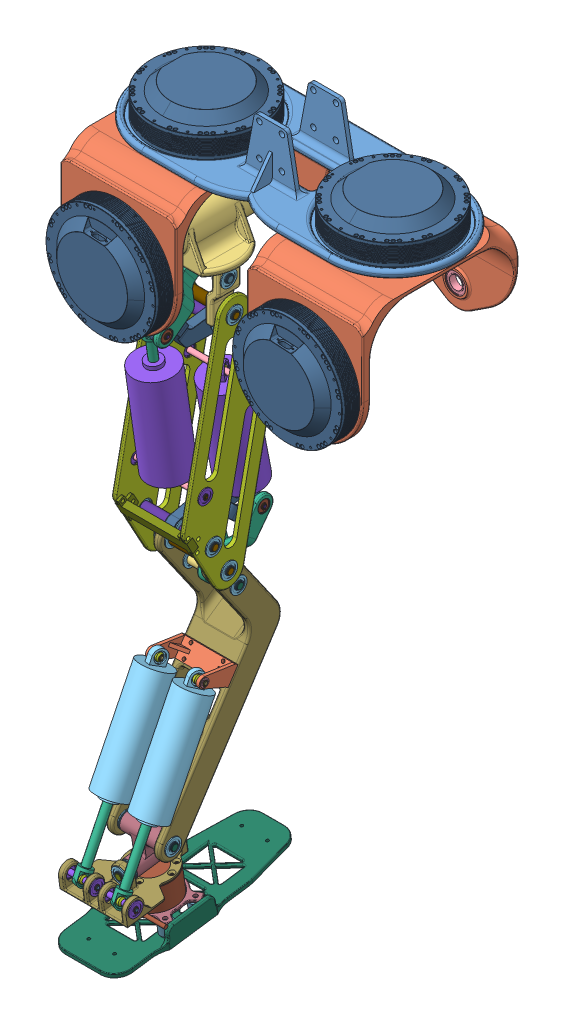
SolidWorks assembly 纯下肢, configuration 默认. Lengths in mm.
Overall size (490 1133.74 383.33).
196 component instances, 46 part files, 330 mates.
Components (placement in the parent):
- 腰部固定座-1: 腰部固定座 [默认] at (0 279.9038 -219.3997) size (490 92.32 200)
- 髋旋转轴-1: 髋旋转轴 [默认] at (-145 260.4038 -219.3997) x (0 0 1) z (-1 0 0) size (243 210 186.66)
- 髋侧摆轴-1: 髋侧摆轴 [默认] at (-145 150.4038 -206.8997) x (-1 0 0) z (0 0 -1) size (125 160 235.8)
- 20mm法兰轴承F63804ZZ-1: 20mm法兰轴承F63804ZZ [默认] at (-145 150.4038 -317.3997) x (0 0 -1) z (0.948831 0.315784 0) size (10 35 35)
- 法兰轴承10_22_6-1: 法兰轴承10_22_6 [默认] at (-190.25 95.4038 -201.6733) x (0 0.630606 0.776103) z (0 0.776103 -0.630606) size (25 6 25)
- 法兰轴承10_22_6-2: 法兰轴承10_22_6 [默认] at (-180.25 45.6778 -206.8997) x (0 -0.265433 0.964129) z (0 0.964129 0.265433) size (25 6 25)
- 法兰轴承10_22_6-3: 法兰轴承10_22_6 [默认] at (-182.25 45.6778 -206.8997) x (0 -0.354717 -0.934974) z (0 0.934974 -0.354717) size (25 6 25)
- 法兰轴承10_22_6-4: 法兰轴承10_22_6 [默认] at (-192.25 95.4038 -201.6733) x (0 -0.95037 0.311121) z (0 -0.311121 -0.95037) size (25 6 25)
- 法兰轴承10_22_6-5: 法兰轴承10_22_6 [默认] at (-99.75 95.4038 -201.6733) x (0 0.630606 0.776103) z (0 -0.776103 0.630606) size (25 6 25)
- 法兰轴承10_22_6-6: 法兰轴承10_22_6 [默认] at (-109.75 45.6778 -206.8997) x (0 -0.265433 0.964129) z (0 -0.964129 -0.265433) size (25 6 25)
- 法兰轴承10_22_6-7: 法兰轴承10_22_6 [默认] at (-107.75 45.6778 -206.8997) x (0 -0.354717 -0.934974) z (0 -0.934974 0.354717) size (25 6 25)
- 法兰轴承10_22_6-8: 法兰轴承10_22_6 [默认] at (-97.75 95.4038 -201.6733) x (0 -0.95037 0.311121) z (0 0.311121 0.95037) size (25 6 25)
- 膝关节U型架-3: 膝关节U型架 [默认] at (-152.25 107.2713 -192.4992) x (1 0 0) z (0 -0.791163 -0.611605) size (56 120 30)
- 法兰轴承10_22_6-9: 法兰轴承10_22_6 [默认] at (-147.75 95.4038 -201.6733) x (0 -0.354389 -0.935098) z (0 0.935098 -0.354389) size (25 6 25)
- 法兰轴承10_22_6-10: 法兰轴承10_22_6 [默认] at (-142.25 95.4038 -201.6733) x (0 -0.969672 -0.244408) z (0 -0.244408 0.969672) size (25 6 25)
- 大腿侧板-1: 大腿侧板 [默认] at (-194.75 -294.2141 -198.324) x (-1 0 0) z (0 0.025223 0.999682) size (6 390 144.2)
- 法兰轴承10_22_6-11: 法兰轴承10_22_6 [默认] at (-196.25 -294.2141 -198.324) x (0 -0.631421 0.77544) z (0 -0.77544 -0.631421) size (25 6 25)
- 法兰轴承5-19-6-1: 法兰轴承5-19-6 [默认] at (-196.25 -176.2424 -161.2878) x (0 -0.967819 -0.251646) z (0 0.251646 -0.967819) size (22 6 22)
- 法兰轴承10_22_6-12: 法兰轴承10_22_6 [默认] at (-196.25 -250.296 -174.4241) x (0 -0.631421 0.77544) z (0 -0.77544 -0.631421) size (25 6 25)
- 法兰轴承5-19-6-2: 法兰轴承5-19-6 [默认] at (-196.25 -73.2936 -243.9107) x (0 -0.631421 0.77544) z (0 -0.77544 -0.631421) size (22 6 22)
- 法兰轴承10_22_6-13: 法兰轴承10_22_6 [默认] at (-196.25 1.7597 -230.7996) x (0 -0.631421 0.77544) z (0 -0.77544 -0.631421) size (25 6 25)
- 法兰轴承10_22_6-14: 法兰轴承10_22_6 [默认] at (-196.25 45.6778 -206.8997) x (0 -0.631421 0.77544) z (0 -0.77544 -0.631421) size (25 6 25)
- 10mm轴114.5mm-1: 10mm轴114.5mm [默认] at (-145 45.6778 -206.8997) x (1 0 0) z (0 0.966924 -0.255065) size (118.9 10 10)
- 大腿侧板-2: 大腿侧板 [默认] at (-89.25 -294.2141 -198.324) x (-1 0 0) z (0 0.025223 0.999682) size (6 390 144.2)
- 法兰轴承10_22_6-19: 法兰轴承10_22_6 [默认] at (-93.75 -294.2141 -198.324) x (0 -0.631421 0.77544) z (0 0.77544 0.631421) size (25 6 25)
- 法兰轴承5-19-6-5: 法兰轴承5-19-6 [默认] at (-93.75 -176.2424 -161.2878) x (0 -0.967819 -0.251646) z (0 -0.251646 0.967819) size (22 6 22)
- 法兰轴承10_22_6-20: 法兰轴承10_22_6 [默认] at (-93.75 -250.296 -174.4241) x (0 -0.631421 0.77544) z (0 0.77544 0.631421) size (25 6 25)
- 法兰轴承5-19-6-6: 法兰轴承5-19-6 [默认] at (-93.75 -73.2936 -243.9107) x (0 -0.631421 0.77544) z (0 0.77544 0.631421) size (22 6 22)
- 法兰轴承10_22_6-21: 法兰轴承10_22_6 [默认] at (-93.75 1.7597 -230.7996) x (0 -0.631421 0.77544) z (0 0.77544 0.631421) size (25 6 25)
- 法兰轴承10_22_6-22: 法兰轴承10_22_6 [默认] at (-93.75 45.6778 -206.8997) x (0 -0.631421 0.77544) z (0 0.77544 0.631421) size (25 6 25)
- 膝关节U型架后侧-3: 膝关节U型架后侧 [默认] at (-152.25 1.6259 -192.216) x (1 0 0) z (0 -0.559181 0.829046) size (38 113.6 87.09)
- 轴承_NSK635-1: 轴承_NSK635 [默认] at (-126 40.3594 -130.4685) x (0 0.759997 0.649927) z (0 -0.649927 0.759997) size (19 6 19)
- 轴承_NSK635-2: 轴承_NSK635 [默认] at (-158 40.3594 -130.4685) x (0 -0.354055 -0.935224) z (0 0.935224 -0.354055) size (19 6 19)
- 轴承_NSK635-3: 轴承_NSK635 [默认] at (-173 40.3594 -130.4685) x (0 0.410059 0.912059) z (0 0.912059 -0.410059) size (19 6 19)
- 轴承_NSK635-4: 轴承_NSK635 [默认] at (-123 40.3594 -130.4685) x (0 0.131283 0.991345) z (0 0.991345 -0.131283) size (19 6 19)
- 法兰轴承10_22_6-27: 法兰轴承10_22_6 [默认] at (-142.25 1.7597 -230.7996) x (0 0.903359 0.428885) z (0 0.428885 -0.903359) size (25 6 25)
- 法兰轴承10_22_6-28: 法兰轴承10_22_6 [默认] at (-147.75 1.7597 -230.7996) x (0 -0.592349 0.805681) z (0 -0.805681 -0.592349) size (25 6 25)
- 法兰轴承10_22_6-29: 法兰轴承10_22_6 [默认] at (-142.25 -250.296 -174.4241) x (0 0.618844 0.785514) z (0 0.785514 -0.618844) size (25 6 25)
- 轴承_NSK635-5: 轴承_NSK635 [默认] at (-158 -263.2782 -281.1374) x (0 0.098206 -0.995166) z (0 0.995166 0.098206) size (19 6 19)
- 轴承_NSK635-6: 轴承_NSK635 [默认] at (-126 -263.2782 -281.1374) x (0 0.098206 -0.995166) z (0 0.995166 0.098206) size (19 6 19)
- 膝关节U型架后侧-4: 膝关节U型架后侧 [默认] at (-152.25 -240.7623 -211.8115) x (1 0 0) z (0 0.74438 -0.667756) size (38 113.6 87.09)
- 法兰轴承10_22_6-30: 法兰轴承10_22_6 [默认] at (-147.75 -250.296 -174.4241) x (0 -0.88858 0.458722) z (0 -0.458722 -0.88858) size (25 6 25)
- 膝关节U型架-4: 膝关节U型架 [默认] at (-152.25 -344.1973 -238.9818) x (1 0 0) z (0 0.601536 0.798846) size (56 120 30)
- 法兰轴承10_22_6-33: 法兰轴承10_22_6 [默认] at (-147.75 -335.1743 -226.9991) x (0 -0.23218 -0.972673) z (0 0.972673 -0.23218) size (25 6 25)
- 法兰轴承10_22_6-34: 法兰轴承10_22_6 [默认] at (-142.25 -335.1743 -226.9991) x (0 -0.932949 -0.360009) z (0 -0.360009 0.932949) size (25 6 25)
- 轴承_NSK635-9: 轴承_NSK635 [默认] at (-173 -263.2782 -281.1374) x (0 0.344761 0.938691) z (0 0.938691 -0.344761) size (19 6 19)
- 轴承_NSK635-10: 轴承_NSK635 [默认] at (-123 -263.2782 -281.1374) x (0 0.010295 0.999947) z (0 0.999947 -0.010295) size (19 6 19)
- 小腿骨-1: 小腿骨 [默认] at (-103.25 -625.3653 -108.2044) x (-1 0 0) z (0 -0.544715 -0.838621) size (83.5 367.8 166.31)
- 法兰轴承10_22_6-37: 法兰轴承10_22_6 [默认] at (-108.75 -335.1743 -226.9991) x (0 0.314255 0.949338) z (0 -0.949338 0.314255) size (25 6 25)
- 法兰轴承10_22_6-38: 法兰轴承10_22_6 [默认] at (-107.75 -294.2141 -198.324) x (0 -0.79401 -0.607905) z (0 -0.607905 0.79401) size (25 6 25)
- 法兰轴承10_22_6-39: 法兰轴承10_22_6 [默认] at (-108.75 -294.2141 -198.324) x (0 0.314255 0.949338) z (0 -0.949338 0.314255) size (25 6 25)
- 法兰轴承10_22_6-40: 法兰轴承10_22_6 [默认] at (-107.75 -335.1743 -226.9991) x (0 -0.79401 -0.607905) z (0 -0.607905 0.79401) size (25 6 25)
- 法兰轴承10_22_6-41: 法兰轴承10_22_6 [默认] at (-182.25 -335.1743 -226.9991) x (0 -0.79401 -0.607905) z (0 0.607905 -0.79401) size (25 6 25)
- 法兰轴承10_22_6-42: 法兰轴承10_22_6 [默认] at (-181.25 -294.2141 -198.324) x (0 0.314255 0.949338) z (0 0.949338 -0.314255) size (25 6 25)
- 法兰轴承10_22_6-43: 法兰轴承10_22_6 [默认] at (-182.25 -294.2141 -198.324) x (0 -0.79401 -0.607905) z (0 0.607905 -0.79401) size (25 6 25)
- 法兰轴承10_22_6-44: 法兰轴承10_22_6 [默认] at (-181.25 -335.1743 -226.9991) x (0 0.314255 0.949338) z (0 0.949338 -0.314255) size (25 6 25)
- 法兰轴承10_22_6-45: 法兰轴承10_22_6 [默认] at (-107.75 -636.5319 -125.3961) x (0 -0.79401 -0.607905) z (0 -0.607905 0.79401) size (25 6 25)
- 法兰轴承10_22_6-46: 法兰轴承10_22_6 [默认] at (-108.75 -636.5319 -125.3961) x (0 0.314255 0.949338) z (0 -0.949338 0.314255) size (25 6 25)
- 法兰轴承10_22_6-47: 法兰轴承10_22_6 [默认] at (-181.25 -636.5319 -125.3961) x (0 0.314255 0.949338) z (0 0.949338 -0.314255) size (25 6 25)
- 法兰轴承10_22_6-48: 法兰轴承10_22_6 [默认] at (-182.25 -636.5319 -125.3961) x (0 -0.79401 -0.607905) z (0 0.607905 -0.79401) size (25 6 25)
- 脚踝交叉转轴套筒-1: 脚踝交叉转轴套筒 [默认] at (-145 -670.4987 -130.2133) x (1 0 0) z (0 -0.140415 0.990093) size (55.5 60.31 62)
- 法兰轴承10_22_6-49: 法兰轴承10_22_6 [默认] at (-121.75 -636.5319 -125.3961) x (0 0.148414 0.988925) z (0 0.988925 -0.148414) size (25 6 25)
- 法兰轴承10_22_6-50: 法兰轴承10_22_6 [默认] at (-168.25 -636.5319 -125.3961) x (0 -0.823067 -0.567944) z (0 0.567944 -0.823067) size (25 6 25)
- 法兰轴承10_22_6-51: 法兰轴承10_22_6 [默认] at (-145 -674.2197 -103.9758) x (-0.579526 -0.80688 -0.114432) z (-0.814954 0.573784 0.081374) size (25 6 25)
- 法兰轴承10_22_6-57: 法兰轴承10_22_6 [默认] at (-145 -666.7777 -156.4507) x (0.812393 0.577334 0.081877) z (-0.583111 0.804344 0.114072) size (25 6 25)
- 10mm轴106.5mm-1: 10mm轴106.5mm [默认] at (-145 95.4038 -201.6733) x (1 0 0) z (0 -0.031617 0.9995) size (110.9 10 10)
- 10mm轴114.5mm-2: 10mm轴114.5mm [默认] at (-145 1.7597 -230.7996) x (1 0 0) z (0 -0.031617 0.9995) size (118.9 10 10)
- 10mm轴114.5mm-3: 10mm轴114.5mm [默认] at (-145 -250.296 -174.4241) x (1 0 0) z (0 -0.031617 0.9995) size (118.9 10 10)
- 10mm轴114.5mm-4: 10mm轴114.5mm [默认] at (-145 -294.2141 -198.324) x (1 0 0) z (0 -0.031617 0.9995) size (118.9 10 10)
- 10mm轴86.5mm-1: 10mm轴86.5mm [默认] at (-145 -335.1743 -226.9991) x (1 0 0) z (0 -0.330259 0.94389) size (90.9 10 10)
- 10mm轴86.5mm-2: 10mm轴86.5mm [默认] at (-145 -636.5319 -125.3961) x (1 0 0) z (0 -0.031617 0.9995) size (90.9 10 10)
- 10mm轴93mm-1: 10mm轴93mm [默认] at (-145 -670.4987 -130.2133) x (0 -0.140415 0.990093) z (-0.999046 -0.043243 -0.006133) size (97.4 10 10)
- 5mm轴56mm-1: 5mm轴56mm [默认] at (-145 40.3594 -130.4685) x (1 0 0) z (0 -0.047055 0.998892) size (59.2 5 5)
- 5mm轴56mm-2: 5mm轴56mm [默认] at (-145 -263.2782 -281.1374) x (1 0 0) z (0 -0.969218 -0.246204) size (59.2 5 5)
- 5mm轴114.5mm-1: 5mm轴114.5mm [默认] at (-145 -176.2424 -161.2878) x (1 0 0) z (0 -0.046931 0.998898) size (117.7 5 5)
- 5mm轴114.5mm-2: 5mm轴114.5mm [默认] at (-145 -73.2936 -243.9107) x (1 0 0) z (0 -0.046931 0.998898) size (117.7 5 5)
- 5mm轴48mm-1: 5mm轴48mm [默认] at (-175 -681.0298 -55.9563) x (1 0 0) z (0 -0.106597 0.994302) size (51.2 5 5)
- 5mm轴48mm-2: 5mm轴48mm [默认] at (-115 -681.0298 -55.9563) x (1 0 0) z (0 0.203949 0.978981) size (51.2 5 5)
- 脚踝推杆上固定座-1: 脚踝推杆上固定座 [默认] at (-145 -454.2866 -219.3263) x (1 0 0) z (0 0.544715 0.838621) size (83.5 34.93 52.93)
- 5mm轴17.25mm-1: 5mm轴17.25mm [默认] at (-110.875 -440.6765 -174.5071) x (1 0 0) z (0 -0.031617 0.9995) size (20.45 5 5)
- 5mm轴17.25mm-2: 5mm轴17.25mm [默认] at (-179.125 -440.6765 -174.5071) x (1 0 0) z (0 -0.999464 0.032733) size (20.45 5 5)
- 法兰轴承5_11_5-1: 法兰轴承5_11_5 [默认] at (-182.75 -440.6765 -174.5071) x (0 0.990767 0.135576) z (0 -0.135576 0.990767) size (12.5 5 12.5)
- 法兰轴承5_11_5-2: 法兰轴承5_11_5 [默认] at (-107.25 -440.6765 -174.5071) x (0 0.231571 -0.972818) z (0 -0.972818 -0.231571) size (12.5 5 12.5)
- 脚踝推杆-1: 脚踝推杆 [默认] at (-175 -590.8973 -100.4128) x (-0.307617 0.420904 0.853353) z (-0.95151 -0.136075 -0.275883) size (50 289 50) (flexible)
  - 脚踝推杆本体-1: 脚踝推杆本体 [默认] at origin size (50 184.5 50)
  - 脚踝推杆伸缩杆-1: 脚踝推杆伸缩杆 [默认] at (0 -86 0) x (-1 0 0) z (0 0 1) size (20 104.5 20)
  - 脚踝推杆球头-1: 脚踝推杆球头 [默认] at (-6.9559 -113.0223 2.2488) x (0.82173 -0.504167 -0.26566) z (0.307617 0 0.95151) size (13 13 9)
  - 脚踝推杆球头-2: 脚踝推杆球头 [默认] at (-7.5682 155.3763 2.4468) x (0.795577 -0.548547 -0.257204) z (0.307617 0 0.95151) size (13 13 9)
- 脚踝推杆-2: 脚踝推杆 [默认] at (-115 -590.8973 -100.4128) x (-0.456371 0.393602 0.798) z (-0.88979 -0.201877 -0.409292) size (50 289 50) (flexible)
  - 脚踝推杆本体-1: 脚踝推杆本体 [默认] at origin size (50 184.5 50)
  - 脚踝推杆伸缩杆-1: 脚踝推杆伸缩杆 [默认] at (0 -86 0) x (-1 0 0) z (0 0 1) size (20 104.5 20)
  - 脚踝推杆球头-1: 脚踝推杆球头 [默认] at (-6.8448 -112.7912 3.5107) x (0.754246 -0.530528 -0.38685) z (0.456371 0 0.88979) size (13 13 9)
  - 脚踝推杆球头-2: 脚踝推杆球头 [默认] at (-7.0773 155.3763 3.6299) x (0.743971 -0.548547 -0.38158) z (0.456371 0 0.88979) size (13 13 9)
- 膝髋推杆-1: 膝髋推杆 [默认] at (-1317.345 -329.4229 96.4698) x (0.141049 0.419648 0.896661) z (-0.989055 0.099352 0.109085) size (174.37 207.64 107.94) (flexible)
  - 膝髋推杆本体-1: 膝髋推杆本体 [默认] at (-128.4703 295.8309 -1190.686) x (0.755997 -0.485294 -0.43927) z (0.295191 -0.346203 0.890509) size (65 181.5 65)
  - 脚踝推杆球头-1: 脚踝推杆球头 [默认] at (-33.4813 413.4712 -1171.9885) x (0.986998 -0.083932 0.137081) z (-0.141049 -0.043308 0.989055) size (13 13 9)
  - 脚踝推杆伸缩杆-1: 脚踝推杆伸缩杆 [默认] at (-136.9986 284.1107 -1192.4154) x (-0.755997 0.485294 0.43927) z (0.295191 -0.346203 0.890509) size (20 104.5 20)
  - 脚踝推杆球头-2: 脚踝推杆球头 [默认] at (-146.5878 258.0336 -1194.9248) x (0.986997 -0.083942 0.13708) z (-0.141049 -0.043308 0.989055) size (13 13 9)
- 膝髋推杆-2: 膝髋推杆 [默认] at (-145.5266 -324.8147 -29.4067) x (0.043782 0.860601 -0.507395) z (-0.991589 0.099352 0.08295) size (216.38 190.11 98.28) (flexible)
  - 膝髋推杆本体-1: 膝髋推杆本体 [默认] at (323.1998 -62.3825 21.4019) x (-0.621633 -0.745576 0.240186) z (-0.065748 -0.255884 -0.964469) size (65 181.5 65)
  - 脚踝推杆球头-1: 脚踝推杆球头 [默认] at (193.5699 24.4942 5.0071) x (0.995432 -0.078977 0.053653) z (-0.043782 0.121798 0.991589) size (13 13 9)
  - 脚踝推杆伸缩杆-1: 脚踝推杆伸缩杆 [默认] at (354.2525 -86.8627 25.7799) x (0.621633 0.745576 -0.240186) z (-0.065748 -0.255884 -0.964469) size (20 104.5 20)
  - 脚踝推杆球头-2: 脚踝推杆球头 [默认] at (368.1521 -109.9327 29.2273) x (0.983046 0.182149 0.021031) z (-0.043782 0.121798 0.991589) size (13 13 9)
- 轴端挡圈GB894-5-1: 轴端挡圈GB894-5 [默认] at (-173 40.3594 -130.4685) x (0 -0.86281 -0.505529) z (-1 0 0) size (6.3 8.28 0.6)
- 轴端挡圈GB894-5-2: 轴端挡圈GB894-5 [默认] at (-116.4 40.3594 -130.4685) x (0 -0.86281 -0.505529) z (-1 0 0) size (6.3 8.28 0.6)
- 轴端挡圈GB894-5-3: 轴端挡圈GB894-5 [默认] at (-87.15 -73.2936 -243.9107) x (0 0.06273 0.998031) z (-1 0 0) size (6.3 8.28 0.6)
- 轴端挡圈GB894-5-4: 轴端挡圈GB894-5 [默认] at (-202.25 -73.2936 -243.9107) x (0 0.06273 0.998031) z (-1 0 0) size (6.3 8.28 0.6)
- 轴端挡圈GB894-5-5: 轴端挡圈GB894-5 [默认] at (-202.25 -176.2424 -161.2878) x (0 -0.221289 0.975208) z (-1 0 0) size (6.3 8.28 0.6)
- 轴端挡圈GB894-5-6: 轴端挡圈GB894-5 [默认] at (-116.4 -263.2782 -281.1374) x (0 0.06273 0.998031) z (-1 0 0) size (6.3 8.28 0.6)
- 轴端挡圈GB894-5-7: 轴端挡圈GB894-5 [默认] at (-87.15 -176.2424 -161.2878) x (0 0.06273 0.998031) z (-1 0 0) size (6.3 8.28 0.6)
- 轴端挡圈GB894-5-8: 轴端挡圈GB894-5 [默认] at (-173.6 -263.2782 -281.1374) x (0 0.449434 -0.893313) z (1 0 0) size (6.3 8.28 0.6)
- 轴端挡圈GB894-5-9: 轴端挡圈GB894-5 [默认] at (-101.65 -440.6765 -174.5071) x (0 0.06273 0.998031) z (-1 0 0) size (6.3 8.28 0.6)
- 轴端挡圈GB894-5-10: 轴端挡圈GB894-5 [默认] at (-169.9 -440.6765 -174.5071) x (0 0.06273 0.998031) z (-1 0 0) size (6.3 8.28 0.6)
- 轴端挡圈GB894-5-11: 轴端挡圈GB894-5 [默认] at (-120.1 -440.6765 -174.5071) x (0 -0.931592 -0.363507) z (1 0 0) size (6.3 8.28 0.6)
- 轴端挡圈GB894-5-12: 轴端挡圈GB894-5 [默认] at (-188.35 -440.6765 -174.5071) x (0 -0.931592 -0.363507) z (1 0 0) size (6.3 8.28 0.6)
- 轴端挡圈GB894-5-13: 轴端挡圈GB894-5 [默认] at (-90.4 -681.0298 -55.9563) x (0 0.062948 0.998017) z (-1 0 0) size (6.3 8.28 0.6)
- 轴端挡圈GB894-5-14: 轴端挡圈GB894-5 [默认] at (-199.6 -681.0298 -55.9563) x (0 -0.931671 -0.363303) z (1 0 0) size (6.3 8.28 0.6)
- 轴端挡圈GB894-5-15: 轴端挡圈GB894-5 [默认] at (-150.4 -681.0298 -55.9563) x (0 0.062948 0.998017) z (-1 0 0) size (6.3 8.28 0.6)
- 轴端挡圈GB894-5-17: 轴端挡圈GB894-5 [默认] at (-140.5144 -681.0298 -55.9563) x (0 -0.123473 0.992348) z (-1 0 0) size (6.3 8.28 0.6)
- 轴端挡圈GB894-10-1: 轴端挡圈GB894-10 [默认] at (-189.25 -636.5319 -125.3961) x (0 -0.931592 -0.363507) z (1 0 0) size (11.5 12.44 1)
- 轴端挡圈GB894-10-2: 轴端挡圈GB894-10 [默认] at (-100.75 -636.5319 -125.3961) x (0 0.06273 0.998031) z (-1 0 0) size (11.5 12.44 1)
- 轴端挡圈GB894-10-3: 轴端挡圈GB894-10 [默认] at (-145 -677.1684 -83.1838) x (-0.667499 -0.737234 -0.104554) z (0 0.140415 -0.990093) size (11.5 12.44 1)
- 轴端挡圈GB894-10-4: 轴端挡圈GB894-10 [默认] at (-145 -663.9694 -176.2526) x (-0.897601 -0.436441 -0.061896) z (0 0.140415 -0.990093) size (11.5 12.44 1)
- 轴端挡圈GB894-10-5: 轴端挡圈GB894-10 [默认] at (-188.25 -335.1743 -226.9991) x (0 0.06273 0.998031) z (-1 0 0) size (11.5 12.44 1)
- 轴端挡圈GB894-10-6: 轴端挡圈GB894-10 [默认] at (-202.25 -294.2141 -198.324) x (0 0.06273 0.998031) z (-1 0 0) size (11.5 12.44 1)
- 轴端挡圈GB894-10-7: 轴端挡圈GB894-10 [默认] at (-202.25 -250.296 -174.4241) x (0 0.06273 0.998031) z (-1 0 0) size (11.5 12.44 1)
- 轴端挡圈GB894-10-8: 轴端挡圈GB894-10 [默认] at (-202.25 45.6778 -206.8997) x (0 0.06273 0.998031) z (-1 0 0) size (11.5 12.44 1)
- 轴端挡圈GB894-10-9: 轴端挡圈GB894-10 [默认] at (-202.25 1.7597 -230.7996) x (0 0.06273 0.998031) z (-1 0 0) size (11.5 12.44 1)
- 轴端挡圈GB894-10-10: 轴端挡圈GB894-10 [默认] at (-198.25 95.4038 -201.6733) x (0 0.06273 0.998031) z (-1 0 0) size (11.5 12.44 1)
- 轴端挡圈GB894-10-11: 轴端挡圈GB894-10 [默认] at (-91.75 95.4038 -201.6733) x (0 -0.931592 -0.363507) z (1 0 0) size (11.5 12.44 1)
- 轴端挡圈GB894-10-12: 轴端挡圈GB894-10 [默认] at (-87.75 45.6778 -206.8997) x (0 -0.931592 -0.363507) z (1 0 0) size (11.5 12.44 1)
- 轴端挡圈GB894-10-13: 轴端挡圈GB894-10 [默认] at (-87.75 1.7597 -230.7996) x (0 -0.931592 -0.363507) z (1 0 0) size (11.5 12.44 1)
- 轴端挡圈GB894-10-14: 轴端挡圈GB894-10 [默认] at (-87.75 -250.296 -174.4241) x (0 -0.931592 -0.363507) z (1 0 0) size (11.5 12.44 1)
- 轴端挡圈GB894-10-15: 轴端挡圈GB894-10 [默认] at (-101.75 -335.1743 -226.9991) x (0 -0.931592 -0.363507) z (1 0 0) size (11.5 12.44 1)
- 轴端挡圈GB894-10-16: 轴端挡圈GB894-10 [默认] at (-87.75 -294.2141 -198.324) x (0 -0.931592 -0.363507) z (1 0 0) size (11.5 12.44 1)
- 20mm法兰轴承F63804ZZ-3: 20mm法兰轴承F63804ZZ [默认] at (145 150.4038 -317.3997) x (0 0 -1) z (0.948831 -0.315784 0) size (10 35 35)
- 髋旋转轴-2: 髋旋转轴 [默认] at (145 260.4038 -219.3997) x (0 0 1) z (-1 0 0) size (243 210 186.66)
- 脚踝-1: 脚踝 [默认] at (-145 -726.934 -138.2169) x (-1 0 0) z (0 0.990093 0.140415) size (117.35 300 99.3) (flexible)
  - 六轴力_力矩传感器-1: 六轴力_力矩传感器 [默认] at origin size (92 76.2 38)
  - 脚踝上支承板-1: 脚踝上支承板 [默认] at (0 0 38) x (1 0 0) z (0 -1 0) size (105 34 134)
  - 脚踝中支承板-1: 脚踝中支承板 [默认] at (0 0 -4) x (1 0 0) z (0 -1 0) size (103.1 6.09 76.22)
  - 橡胶减震柱2015DE06-1: 橡胶减震柱2015DE06 [默认] at (41.1362 -23.75 -9.5) x (-0.313496 0.949589 0) z (-0.949589 -0.313496 0) size (20 15 20)
  - 橡胶减震柱2015DE06-2: 橡胶减震柱2015DE06 [默认] at (41.1362 23.75 -9.5) x (-0.21278 0.9771 0) z (-0.9771 -0.21278 0) size (20 15 20)
  - 橡胶减震柱2015DE06-3: 橡胶减震柱2015DE06 [默认] at (-41.1362 -23.75 -9.5) x (-0.313496 0.949589 0) z (-0.949589 -0.313496 0) size (20 15 20)
  - 橡胶减震柱2015DE06-4: 橡胶减震柱2015DE06 [默认] at (-41.1362 23.75 -9.5) x (-0.313496 0.949589 0) z (-0.949589 -0.313496 0) size (20 15 20)
  - 脚掌-1: 脚掌 [默认] at (0 -185 -25) x (1 0 0) z (0 -1 0) size (117.35 30 300)
  - 法兰轴承10_22_6-1: 法兰轴承10_22_6 [默认] at (0 40.5 57) size (25 6 25)
  - 法兰轴承5-19-6-1: 法兰轴承5-19-6 [默认] at (48 75 57) x (0 -0.990093 -0.140417) z (0 -0.140417 0.990093) size (22 6 22)
  - 法兰轴承5-19-6-2: 法兰轴承5-19-6 [默认] at (-12 75 57) x (0 -0.990093 -0.140417) z (0 -0.140417 0.990093) size (22 6 22)
  - 法兰轴承5-19-6-3: 法兰轴承5-19-6 [默认] at (12 75 57) x (0 0.717248 -0.696818) z (0 0.696818 0.717248) size (22 6 22)
  - 法兰轴承5-19-6-4: 法兰轴承5-19-6 [默认] at (-48 75 57) x (0 -0.340246 0.940337) z (0 -0.940337 -0.340246) size (22 6 22)
  - 法兰轴承10_22_6-2: 法兰轴承10_22_6 [默认] at (0 39.5 57) x (-0.453599 0 -0.891206) z (-0.891206 0 0.453599) size (25 6 25)
  - 法兰轴承10_22_6-3: 法兰轴承10_22_6 [默认] at (0 -39.5 57) size (25 6 25)
  - 法兰轴承10_22_6-4: 法兰轴承10_22_6 [默认] at (0 -40.5 57) x (-0.837169 0 -0.546944) z (-0.546944 0 0.837169) size (25 6 25)
- 大腿侧板柱-5: 大腿侧板柱 [默认] at (-145 -15.0312 -262.7067) x (-1 0 0) z (0 0.878361 0.477998) size (111.5 20 40)
- 大腿侧板柱-6: 大腿侧板柱 [默认] at (-145 -233.5051 -142.517) x (1 0 0) z (0 0.878361 0.477998) size (111.5 20 40)
- 10mm轴套42.5mm-1: 10mm轴套42.5mm [默认] at (-136.25 1.7597 -230.7996) x (0 -1 0) z (0 0 1) size (15 42.5 15)
- 10mm轴套42.5mm-2: 10mm轴套42.5mm [默认] at (-196.25 1.7597 -230.7996) x (0 -1 0) z (0 0 1) size (15 42.5 15)
- 10mm轴套42.5mm-3: 10mm轴套42.5mm [默认] at (-136.25 -250.296 -174.4241) x (0 -1 0) z (0 0 1) size (15 42.5 15)
- 10mm轴套42.5mm-4: 10mm轴套42.5mm [默认] at (-196.25 -250.296 -174.4241) x (0 -0.999841 0.017855) z (0 0.017855 0.999841) size (15 42.5 15)
- 10mm轴套60.5mm-1: 10mm轴套60.5mm [默认] at (-176.25 45.6778 -206.8997) x (0 0.296961 0.95489) z (0 0.95489 -0.296961) size (15 60.5 15)
- 10mm轴套60.5mm-2: 10mm轴套60.5mm [默认] at (-175.25 -294.2141 -198.324) x (0 0.016165 -0.999869) z (0 -0.999869 -0.016165) size (15 60.5 15)
- 10mm轴套30.5mm-1: 10mm轴套30.5mm [默认] at (-184.25 95.4038 -201.6733) x (0 -1 0) z (0 0 1) size (15 30.5 15)
- 10mm轴套30.5mm-2: 10mm轴套30.5mm [默认] at (-136.25 95.4038 -201.6733) x (0 -1 0) z (0 0 1) size (15 30.5 15)
- 10mm轴套8mm-1: 10mm轴套8mm [默认] at (-196.25 -294.2141 -198.324) x (0 -1 0) z (0 0 1) size (15 8 15)
- 10mm轴套8mm-2: 10mm轴套8mm [默认] at (-101.75 -294.2141 -198.324) x (0 -1 0) z (0 0 1) size (15 8 15)
- 10mm轴套8mm-3: 10mm轴套8mm [默认] at (-196.25 45.6778 -206.8997) x (0 -1 0) z (0 0 1) size (15 8 15)
- 10mm轴套8mm-4: 10mm轴套8mm [默认] at (-101.75 45.6778 -206.8997) x (0 -1 0) z (0 0 1) size (15 8 15)
- 10mm轴套21.5mm-1: 10mm轴套21.5mm [默认] at (-175.25 -335.1743 -226.9991) x (0 -1 0) z (0 0 1) size (15 21.5 15)
- 10mm轴套21.5mm-2: 10mm轴套21.5mm [默认] at (-136.25 -335.1743 -226.9991) x (0 -1 0) z (0 0 1) size (15 21.5 15)
- 5mm轴套46.75mm-1: 5mm轴套46.75mm [默认] at (-140.5 -73.2936 -243.9107) x (0 -1 0) z (0 0 1) size (8 46.75 8)
- 5mm轴套46.75mm-2: 5mm轴套46.75mm [默认] at (-140.5 -176.2424 -161.2878) x (0 0.730668 -0.682733) z (0 -0.682733 -0.730668) size (8 46.75 8)
- 5mm轴套46.75mm-3: 5mm轴套46.75mm [默认] at (-196.25 -176.2424 -161.2878) x (0 -1 0) z (0 0 1) size (8 46.75 8)
- 5mm轴套46.75mm-4: 5mm轴套46.75mm [默认] at (-196.25 -73.2936 -243.9107) x (0 -0.999066 0.04322) z (0 0.04322 0.999066) size (8 46.75 8)
- 10mm垫片1mm-1: 10mm垫片1mm [默认] at (-145 -675.0622 -98.0352) x (1 0 0) z (0 -0.990093 -0.140415) size (15 1 15)
- 10mm垫片1mm-2: 10mm垫片1mm [默认] at (-175.25 -636.5319 -125.3961) x (0 -1 0) z (0 0 1) size (15 1 15)
- 10mm垫片1mm-3: 10mm垫片1mm [默认] at (-115.75 -636.5319 -125.3961) x (0 -1 0) z (0 0 1) size (15 1 15)
- 10mm垫片1mm-4: 10mm垫片1mm [默认] at (-145 -665.7948 -163.3814) x (1 0 0) z (0 -0.990093 -0.140415) size (15 1 15)
- 5mm轴套3mm-1: 5mm轴套3mm [默认] at (-126 -263.2782 -281.1374) x (0 -1 0) z (0 0 1) size (8 3 8)
- 5mm轴套3mm-2: 5mm轴套3mm [默认] at (-164 -263.2782 -281.1374) x (0 1 0) z (0 0 1) size (8 3 8)
- 5mm轴套3mm-3: 5mm轴套3mm [默认] at (-126 40.3594 -130.4685) x (0 -1 0) z (0 0 1) size (8 3 8)
- 5mm轴套3mm-4: 5mm轴套3mm [默认] at (-167 40.3594 -130.4685) x (0 -1 0) z (0 0 1) size (8 3 8)
- 5mm轴套8.5mm-1: 5mm轴套8.5mm [默认] at (-132 -263.2782 -281.1374) x (0 1 0) z (0 0 1) size (8 8.5 8)
- 5mm轴套8.5mm-2: 5mm轴套8.5mm [默认] at (-149.5 -263.2782 -281.1374) x (0 1 0) z (0 0 1) size (8 8.5 8)
- 5mm轴套8.5mm-3: 5mm轴套8.5mm [默认] at (-149.5 40.3594 -130.4685) x (0 1 0) z (0 0 1) size (8 8.5 8)
- 5mm轴套8.5mm-4: 5mm轴套8.5mm [默认] at (-132 40.3594 -130.4685) x (0 1 0) z (0 0 1) size (8 8.5 8)
- 5mm轴套13.5mm-1: 5mm轴套13.5mm [默认] at (-195.4256 -681.0298 -55.9563) x (0 -1 0.000002) z (0 0.000002 1) size (8 13.5 8)
- 5mm轴套13.5mm-2: 5mm轴套13.5mm [默认] at (-157 -681.0298 -55.9563) x (0 1 -0.000002) z (0 0.000002 1) size (8 13.5 8)
- 5mm轴套13.5mm-3: 5mm轴套13.5mm [默认] at (-119.5 -681.0298 -55.9563) x (0 0.999945 0.010515) z (0 -0.010515 0.999945) size (8 13.5 8)
- 5mm轴套13.5mm-4: 5mm轴套13.5mm [默认] at (-97 -681.0298 -55.9563) x (0 1 -0.000002) z (0 0.000002 1) size (8 13.5 8)
- 5mm轴套3.25mm-1: 5mm轴套3.25mm [默认] at (-110.5 -440.6765 -174.5071) x (0 -1 0) z (0 0 1) size (8 3.25 8)
- 5mm轴套3.25mm-2: 5mm轴套3.25mm [默认] at (-182.75 -440.6765 -174.5071) x (0 -1 0) z (0 0 1) size (8 3.25 8)
- B1电机模型-1: B1电机模型 [默认] at (315.635 148.0251 -148.1152) x (0 0 1) z (-0.998427 0.056065 0) size (57.67 170.5 170.5)
- B1电机模型-2: B1电机模型 [默认] at (25.635 148.0251 -148.1152) x (0 0 1) z (-0.998427 0.056065 0) size (57.67 170.5 170.5)
- B1电机模型-3: B1电机模型 [默认] at (136.9038 220.1883 -389.8591) x (0 1 0) z (0.005306 0 0.999986) size (57.67 170.5 170.5)
- B1电机模型-4: B1电机模型 [默认] at (-153.0962 220.1883 -389.8591) x (0 1 0) z (0.005306 0 0.999986) size (57.67 170.5 170.5)
Mates (geometry in assembly coordinates):
- 重合1: coincident anti-aligned: plane of 腰部固定座v3.0.3-1 through (-80 279.9038 -219.3997) normal (0 1 0); plane of B1电机模型-220923.STEP-1/B1________-220923.STEP.STEP-1/11UXMR1_DVUR40_HOSR1_BASR1.STEP.STEP-1 through (-203.1424 0 9.0983) normal (0 -1 0)
- 同心1: concentric anti-aligned: cylinder of B1电机模型-220923.STEP-1/B1________-220923.STEP.STEP-1/11UXMR1_DVUR40_BCVR1_BASR1.STEP.STEP-1 through (-145 -42.2 0) axis (0 -1 0) radius 85.25; cylinder of 腰部固定座v3.0.3-1 through (-145 285.9038 -219.3997) axis (0 1 0) radius 65
- 同心2: concentric anti-aligned: cylinder of 腰部固定座v3.0.3-1 through (-198.352 273.9028 -158.1206) axis (0 1 0) radius 2.75; cylinder of B1电机模型-220923.STEP-1/B1________-220923.STEP.STEP-1/11UXMR1_DVUR40_HOSR1_BASR1.STEP.STEP-1 through (-198.352 0 61.2791) axis (0 -1 0) radius 2.5
- 同心7: concentric anti-aligned: cylinder of 髋侧摆轴v3.0.5-1 through (-145 150.4038 -315.8997) axis (0 0 -1) radius 10; cylinder of 20mm法兰轴承F63804ZZ-1 through (-145 150.4038 -317.3997) axis (0 0 1) radius 10
- 同心8: concentric aligned: cylinder of 髋侧摆轴v3.0.5-1 through (-196.75 95.4038 -201.6733) axis (1 0 0) radius 11; cylinder of 法兰轴承10_22_6-1 through (-185.6387 95.4038 -201.6733) axis (1 0 0) radius 11
- 重合6: coincident anti-aligned: plane of 髋侧摆轴v3.0.5-1 through (-185.75 80.4038 -333.7007) normal (1 0 0); plane of 法兰轴承10_22_6-1 through (-185.75 95.4038 -201.6733) normal (-1 0 0)
- 重合7: coincident anti-aligned: plane of 髋侧摆轴v3.0.5-1 through (-196.75 150.4038 -206.8997) normal (-1 0 0); plane of 法兰轴承10_22_6-4 through (-196.75 95.4038 -201.6733) normal (1 0 0)
- 同心9: concentric anti-aligned: cylinder of 髋侧摆轴v3.0.5-1 through (-196.75 95.4038 -201.6733) axis (1 0 0) radius 11; cylinder of 法兰轴承10_22_6-4 through (-196.8613 95.4038 -201.6733) axis (-1 0 0) radius 11
- 同心10: concentric anti-aligned: cylinder of 髋侧摆轴v3.0.5-1 through (-196.75 45.6778 -206.8997) axis (1 0 0) radius 11; cylinder of 法兰轴承10_22_6-3 through (-186.8613 45.6778 -206.8997) axis (-1 0 0) radius 11
- 重合8: coincident anti-aligned: plane of 髋侧摆轴v3.0.5-1 through (-186.75 30.4038 -333.7007) normal (-1 0 0); plane of 法兰轴承10_22_6-3 through (-186.75 45.6778 -206.8997) normal (1 0 0)
- 同心11: concentric aligned: cylinder of 髋侧摆轴v3.0.5-1 through (-196.75 45.6778 -206.8997) axis (1 0 0) radius 11; cylinder of 法兰轴承10_22_6-2 through (-175.6387 45.6778 -206.8997) axis (1 0 0) radius 11
- 重合9: coincident anti-aligned: plane of 髋侧摆轴v3.0.5-1 through (-175.75 30.4038 -333.7007) normal (1 0 0); plane of 法兰轴承10_22_6-2 through (-175.75 45.6778 -206.8997) normal (-1 0 0)
- 同心12: concentric anti-aligned: cylinder of 膝关节U型架-3 through (-157.75 95.4038 -201.6733) axis (1 0 0) radius 11; cylinder of 法兰轴承10_22_6-9 through (-152.3613 95.4038 -201.6733) axis (-1 0 0) radius 11
- 重合10: coincident anti-aligned: plane of 膝关节U型架-3 through (-152.25 68.2463 -191.0682) normal (-1 0 0); plane of 法兰轴承10_22_6-9 through (-152.25 95.4038 -201.6733) normal (1 0 0)
- 同心13: concentric aligned: cylinder of 膝关节U型架-3 through (-157.75 95.4038 -201.6733) axis (1 0 0) radius 11; cylinder of 法兰轴承10_22_6-10 through (-137.6387 95.4038 -201.6733) axis (1 0 0) radius 11
- 重合11: coincident anti-aligned: plane of 膝关节U型架-3 through (-137.75 83.5364 -210.8473) normal (1 0 0); plane of 法兰轴承10_22_6-10 through (-137.75 95.4038 -201.6733) normal (-1 0 0)
- 同心14: concentric anti-aligned: cylinder of 法兰轴承10_22_6-4 through (-196.75 95.4038 -201.6733) axis (-1 0 0) radius 12.5; cylinder of 膝关节U型架-3 through (-157.75 95.4038 -201.6733) axis (1 0 0) radius 11
- 宽度1: width anti-aligned: plane of 膝关节U型架-3 through (-152.25 68.2463 -191.0682) normal (-1 0 0); plane of 髋侧摆轴v3.0.5-1 through (-137.75 83.5364 -210.8473) normal (1 0 0); plane of 膝关节U型架-3 through (-185.75 80.4038 -333.7007) normal (1 0 0); plane of 髋侧摆轴v3.0.5-1 through (-104.25 80.4038 -333.7007) normal (-1 0 0)
- 重合12: coincident anti-aligned: plane of 大腿侧板-1 through (-200.75 -294.2141 -198.324) normal (-1 0 0); plane of 法兰轴承10_22_6-11 through (-200.75 -294.2141 -198.324) normal (1 0 0)
- 同心16: concentric anti-aligned: cylinder of 大腿侧板-1 through (-200.75 -176.2424 -161.2878) axis (1 0 0) radius 9.5; cylinder of 法兰轴承5-19-6-1 through (-200.8613 -176.2424 -161.2878) axis (-1 0 0) radius 9.5
- 重合13: coincident anti-aligned: plane of 大腿侧板-1 through (-200.75 -294.2141 -198.324) normal (-1 0 0); plane of 法兰轴承5-19-6-1 through (-200.75 -176.2424 -161.2878) normal (1 0 0)
- 同心17: concentric anti-aligned: cylinder of 大腿侧板-1 through (-200.75 -250.296 -174.4241) axis (1 0 0) radius 11; cylinder of 法兰轴承10_22_6-12 through (-200.8613 -250.296 -174.4241) axis (-1 0 0) radius 11
- 重合14: coincident anti-aligned: plane of 大腿侧板-1 through (-200.75 -294.2141 -198.324) normal (-1 0 0); plane of 法兰轴承10_22_6-12 through (-200.75 -250.296 -174.4241) normal (1 0 0)
- 同心181: concentric anti-aligned: cylinder of 大腿侧板-1 through (-200.75 -73.2936 -243.9107) axis (1 0 0) radius 9.5; cylinder of 法兰轴承5-19-6-2 through (-200.8613 -73.2936 -243.9107) axis (-1 0 0) radius 9.5
- 同心191: concentric anti-aligned: cylinder of 大腿侧板-1 through (-200.75 1.7597 -230.7996) axis (1 0 0) radius 11; cylinder of 法兰轴承10_22_6-13 through (-200.8613 1.7597 -230.7996) axis (-1 0 0) radius 11
- 同心201: concentric anti-aligned: cylinder of 大腿侧板-1 through (-200.75 45.6778 -206.8997) axis (1 0 0) radius 11; cylinder of 法兰轴承10_22_6-14 through (-200.8613 45.6778 -206.8997) axis (-1 0 0) radius 11
- 重合151: coincident anti-aligned: plane of 大腿侧板-1 through (-200.75 -294.2141 -198.324) normal (-1 0 0); plane of 法兰轴承10_22_6-14 through (-200.75 45.6778 -206.8997) normal (1 0 0)
- 重合161: coincident anti-aligned: plane of 大腿侧板-1 through (-200.75 -294.2141 -198.324) normal (-1 0 0); plane of 法兰轴承10_22_6-13 through (-200.75 1.7597 -230.7996) normal (1 0 0)
- 重合171: coincident anti-aligned: plane of 大腿侧板-1 through (-200.75 -294.2141 -198.324) normal (-1 0 0); plane of 法兰轴承5-19-6-2 through (-200.75 -73.2936 -243.9107) normal (1 0 0)
- 同心211: concentric aligned: cylinder of 法兰轴承10_22_6-2 through (-175.6387 45.6778 -206.8997) axis (1 0 0) radius 5; cylinder of 10mm轴114.5mm-1 through (-85.55 45.6778 -206.8997) axis (1 0 0) radius 5
- 宽度21: width anti-aligned: plane of 10mm轴114.5mm-1 through (-204.45 45.6778 -206.8997) normal (-1 0 0); plane of 髋侧摆轴v3.0.5-1 through (-85.55 45.6778 -206.8997) normal (1 0 0); plane of 10mm轴114.5mm-1 through (-103.25 30.4038 -333.7007) normal (1 0 0); plane of 髋侧摆轴v3.0.5-1 through (-186.75 30.4038 -333.7007) normal (-1 0 0)
- 平行11: parallel anti-aligned: plane of 髋侧摆轴v3.0.5-1 through (-186.75 30.4038 -333.7007) normal (-1 0 0); plane of 大腿侧板-1 through (-194.75 -294.2141 -198.324) normal (1 0 0)
- 同心231: concentric anti-aligned: cylinder of 法兰轴承10_22_6-14 through (-200.8613 45.6778 -206.8997) axis (-1 0 0) radius 5; cylinder of 10mm轴114.5mm-1 through (-85.55 45.6778 -206.8997) axis (1 0 0) radius 5
- 重合191: coincident aligned: plane of 法兰轴承10_22_6-14 through (-202.25 41.5735 -201.8593) normal (-1 0 0); plane of 10mm轴114.5mm-1 through (-202.25 45.6778 -206.8997) normal (-1 0 0)
- 同心241: concentric anti-aligned: cylinder of 膝关节U型架后侧-3 through (-132 40.3594 -130.4685) axis (1 0 0) radius 9.5; cylinder of 轴承_NSK635-1 through (-130.6113 40.3594 -130.4685) axis (-1 0 0) radius 9.5
- 重合211: coincident anti-aligned: plane of 膝关节U型架后侧-3 through (-158 40.3594 -130.4685) normal (-1 0 0); plane of 轴承_NSK635-2 through (-158 37.527 -137.9503) normal (1 0 0)
- 同心251: concentric aligned: cylinder of 膝关节U型架后侧-3 through (-158 40.3594 -130.4685) axis (-1 0 0) radius 9.5; cylinder of 轴承_NSK635-2 through (-162.6113 40.3594 -130.4685) axis (-1 0 0) radius 9.5
- 同心261: concentric aligned: cylinder of 膝关节U型架-3 through (-123 40.3594 -130.4685) axis (1 0 0) radius 9.5; cylinder of 轴承_NSK635-4 through (-118.3887 40.3594 -130.4685) axis (1 0 0) radius 9.5
- 重合231: coincident anti-aligned: plane of 膝关节U型架-3 through (-123 40.3594 -130.4685) normal (1 0 0); plane of 轴承_NSK635-4 through (-123 41.4097 -122.5378) normal (-1 0 0)
- 同心271: concentric anti-aligned: cylinder of 膝关节U型架-3 through (-167 40.3594 -130.4685) axis (-1 0 0) radius 9.5; cylinder of 轴承_NSK635-3 through (-168.3887 40.3594 -130.4685) axis (1 0 0) radius 9.5
- 重合241: coincident anti-aligned: plane of 膝关节U型架-3 through (-167 40.3594 -130.4685) normal (-1 0 0); plane of 轴承_NSK635-3 through (-167 44.255 -121.804) normal (1 0 0)
- 重合251: coincident anti-aligned: plane of 膝关节U型架后侧-3 through (-132 40.3594 -130.4685) normal (1 0 0); plane of 轴承_NSK635-1 through (-132 47.5794 -124.2942) normal (-1 0 0)
- 同心291: concentric anti-aligned: cylinder of 膝关节U型架后侧-3 through (-183.3627 1.7597 -230.7996) axis (1 0 0) radius 11; cylinder of 法兰轴承10_22_6-28 through (-152.3613 1.7597 -230.7996) axis (-1 0 0) radius 11
- 同心301: concentric aligned: cylinder of 膝关节U型架后侧-3 through (-183.3627 1.7597 -230.7996) axis (1 0 0) radius 11; cylinder of 法兰轴承10_22_6-27 through (-137.6387 1.7597 -230.7996) axis (1 0 0) radius 11
- 重合261: coincident anti-aligned: plane of 膝关节U型架后侧-3 through (-152.25 5.3456 -161.9643) normal (-1 0 0); plane of 法兰轴承10_22_6-28 through (-152.25 1.7597 -230.7996) normal (1 0 0)
- 重合271: coincident anti-aligned: plane of 膝关节U型架后侧-3 through (-137.75 -11.2353 -173.148) normal (1 0 0); plane of 法兰轴承10_22_6-27 through (-137.75 1.7597 -230.7996) normal (-1 0 0)
- 同心321: concentric anti-aligned: cylinder of 轴承_NSK635-6 through (-130.6113 -263.2782 -281.1374) axis (-1 0 0) radius 9.5; cylinder of 膝关节U型架后侧-4 through (-132 -263.2782 -281.1374) axis (1 0 0) radius 9.5
- 重合281: coincident anti-aligned: plane of 轴承_NSK635-5 through (-158 -262.4926 -289.0987) normal (1 0 0); plane of 膝关节U型架后侧-4 through (-158 -263.2782 -281.1374) normal (-1 0 0)
- 同心331: concentric aligned: cylinder of 轴承_NSK635-5 through (-162.6113 -263.2782 -281.1374) axis (-1 0 0) radius 9.5; cylinder of 膝关节U型架后侧-4 through (-158 -263.2782 -281.1374) axis (-1 0 0) radius 9.5
- 重合291: coincident anti-aligned: plane of 轴承_NSK635-6 through (-132 -262.3452 -290.5914) normal (-1 0 0); plane of 膝关节U型架后侧-4 through (-132 -263.2782 -281.1374) normal (1 0 0)
- 同心341: concentric anti-aligned: cylinder of 膝关节U型架后侧-4 through (-183.3627 -250.296 -174.4241) axis (1 0 0) radius 11; cylinder of 法兰轴承10_22_6-30 through (-152.3613 -250.296 -174.4241) axis (-1 0 0) radius 11
- 同心351: concentric aligned: cylinder of 法兰轴承10_22_6-29 through (-137.6387 -250.296 -174.4241) axis (1 0 0) radius 11; cylinder of 膝关节U型架后侧-4 through (-183.3627 -250.296 -174.4241) axis (1 0 0) radius 11
- 重合301: coincident anti-aligned: plane of 膝关节U型架后侧-4 through (-152.25 -236.9967 -242.0575) normal (-1 0 0); plane of 法兰轴承10_22_6-30 through (-152.25 -250.296 -174.4241) normal (1 0 0)
- 重合311: coincident anti-aligned: plane of 法兰轴承10_22_6-29 through (-137.75 -250.296 -174.4241) normal (-1 0 0); plane of 膝关节U型架后侧-4 through (-137.75 -223.6416 -227.1699) normal (1 0 0)
- 宽度41: width anti-aligned: plane of 膝关节U型架后侧-4 through (-156 -247.013 -253.2232) normal (1 0 0); plane of 大腿侧板-1 through (-134 -263.707 -271.8327) normal (-1 0 0); plane of 膝关节U型架后侧-4 through (-200.75 -294.2141 -198.324) normal (-1 0 0); plane of 大腿侧板-2 through (-89.25 -294.2141 -198.324) normal (1 0 0)
- 同心411: concentric anti-aligned: cylinder of 膝关节U型架-4 through (-157.75 -335.1743 -226.9991) axis (1 0 0) radius 11; cylinder of 法兰轴承10_22_6-33 through (-152.3613 -335.1743 -226.9991) axis (-1 0 0) radius 11
- 重合361: coincident anti-aligned: plane of 膝关节U型架-4 through (-152.25 -306.1801 -230.0548) normal (-1 0 0); plane of 法兰轴承10_22_6-33 through (-152.25 -335.1743 -226.9991) normal (1 0 0)
- 同心421: concentric aligned: cylinder of 膝关节U型架-4 through (-157.75 -335.1743 -226.9991) axis (1 0 0) radius 11; cylinder of 法兰轴承10_22_6-34 through (-137.6387 -335.1743 -226.9991) axis (1 0 0) radius 11
- 重合371: coincident anti-aligned: plane of 膝关节U型架-4 through (-137.75 -326.1513 -215.0164) normal (1 0 0); plane of 法兰轴承10_22_6-34 through (-137.75 -335.1743 -226.9991) normal (-1 0 0)
- 同心431: concentric aligned: cylinder of 膝关节U型架-4 through (-123 -263.2782 -281.1374) axis (1 0 0) radius 9.5; cylinder of 轴承_NSK635-10 through (-118.3887 -263.2782 -281.1374) axis (1 0 0) radius 9.5
- 重合381: coincident anti-aligned: plane of 膝关节U型架-4 through (-123 -263.2782 -281.1374) normal (1 0 0); plane of 轴承_NSK635-10 through (-123 -263.1958 -273.1378) normal (-1 0 0)
- 同心441: concentric anti-aligned: cylinder of 膝关节U型架-4 through (-167 -263.2782 -281.1374) axis (-1 0 0) radius 9.5; cylinder of 轴承_NSK635-9 through (-168.3887 -263.2782 -281.1374) axis (1 0 0) radius 9.5
- 重合391: coincident anti-aligned: plane of 膝关节U型架-4 through (-167 -263.2782 -281.1374) normal (-1 0 0); plane of 轴承_NSK635-9 through (-167 -260.003 -272.2198) normal (1 0 0)
- 宽度51: width aligned: plane of 膝关节U型架后侧-4 through (-156 -247.013 -253.2232) normal (1 0 0); plane of 膝关节U型架-4 through (-134 -263.707 -271.8327) normal (-1 0 0); plane of 膝关节U型架后侧-4 through (-117 -289.6041 -242.5367) normal (1 0 0); plane of 膝关节U型架-4 through (-173 -254.2552 -269.1547) normal (-1 0 0)
- 同心541: concentric aligned: cylinder of 小腿骨-1 through (-113.25 -636.5319 -125.3961) axis (1 0 0) radius 11; cylinder of 法兰轴承10_22_6-45 through (-103.1387 -636.5319 -125.3961) axis (1 0 0) radius 11
- 重合481: coincident anti-aligned: plane of 小腿骨-1 through (-103.25 -647.6986 -142.5878) normal (1 0 0); plane of 法兰轴承10_22_6-45 through (-103.25 -636.5319 -125.3961) normal (-1 0 0)
- 重合491: coincident anti-aligned: plane of 小腿骨-1 through (-113.25 -622.54 -158.9293) normal (-1 0 0); plane of 法兰轴承10_22_6-46 through (-113.25 -636.5319 -125.3961) normal (1 0 0)
- 同心551: concentric anti-aligned: cylinder of 小腿骨-1 through (-113.25 -636.5319 -125.3961) axis (1 0 0) radius 11; cylinder of 法兰轴承10_22_6-46 through (-113.3613 -636.5319 -125.3961) axis (-1 0 0) radius 11
- 重合501: coincident anti-aligned: plane of 小腿骨-1 through (-103.25 -647.6986 -142.5878) normal (1 0 0); plane of 法兰轴承10_22_6-40 through (-103.25 -335.1743 -226.9991) normal (-1 0 0)
- 重合511: coincident anti-aligned: plane of 小腿骨-1 through (-103.25 -647.6986 -142.5878) normal (1 0 0); plane of 法兰轴承10_22_6-38 through (-103.25 -294.2141 -198.324) normal (-1 0 0)
- 同心581: concentric aligned: cylinder of 小腿骨-1 through (-94.25 -335.1743 -226.9991) axis (-1 0 0) radius 11; cylinder of 法兰轴承10_22_6-37 through (-113.3613 -335.1743 -226.9991) axis (-1 0 0) radius 11
- 同心591: concentric aligned: cylinder of 小腿骨-1 through (-94.25 -294.2141 -198.324) axis (-1 0 0) radius 11; cylinder of 法兰轴承10_22_6-39 through (-113.3613 -294.2141 -198.324) axis (-1 0 0) radius 11
- 重合521: coincident anti-aligned: plane of 小腿骨-1 through (-113.25 -302.9412 -150.1126) normal (-1 0 0); plane of 法兰轴承10_22_6-37 through (-113.25 -335.1743 -226.9991) normal (1 0 0)
- 重合531: coincident anti-aligned: plane of 小腿骨-1 through (-113.25 -302.9412 -150.1126) normal (-1 0 0); plane of 法兰轴承10_22_6-39 through (-113.25 -294.2141 -198.324) normal (1 0 0)
- 宽度61: width anti-aligned: plane of 大腿侧板-2 through (-95.25 -294.2141 -198.324) normal (-1 0 0); plane of 小腿骨-1 through (-194.75 -294.2141 -198.324) normal (1 0 0); plane of 大腿侧板-1 through (-176.75 -302.9412 -150.1126) normal (1 0 0); plane of 小腿骨-1 through (-113.25 -302.9412 -150.1126) normal (-1 0 0)
- 同心621: concentric anti-aligned: cylinder of 脚踝交叉转轴套筒-1 through (-145 -674.8515 -99.5204) axis (0 0.140415 -0.990093) radius 11; cylinder of 法兰轴承10_22_6-51 through (-145 -674.8672 -99.4102) axis (0 -0.140415 0.990093) radius 11
- 重合541: coincident anti-aligned: plane of 脚踝交叉转轴套筒-1 through (-145 -674.8515 -99.5204) normal (0 -0.140415 0.990093); plane of 法兰轴承10_22_6-51 through (-145 -674.8515 -99.5204) normal (0 0.140415 -0.990093)
- 同心631: concentric aligned: cylinder of 脚踝交叉转轴套筒-1 through (-145 -572.1642 131.3677) axis (0 -0.54068 -0.841228) radius 11; cylinder of 法兰轴承10_22_6-52 through (-223.3366 -845.0941 -253.5159) axis (-0.142377 -0.448627 -0.882305) radius 11
- 同心661: concentric anti-aligned: cylinder of 脚掌v3.0.1-1 through (-219.8238 -848.6865 -332.6077) axis (-0.219476 0 -0.975618) radius 11; cylinder of 法兰轴承10_22_6-54 through (-237.3574 -848.6865 -410.5485) axis (0.219476 0 0.975618) radius 11
- 重合581: coincident anti-aligned: plane of 脚掌v3.0.1-1 through (-237.3819 -848.6865 -410.6571) normal (0.219476 0 0.975618); plane of 法兰轴承10_22_6-54 through (-237.3819 -848.6865 -410.6571) normal (-0.219476 0 -0.975618)
- 同心671: concentric aligned: cylinder of 脚掌v3.0.1-1 through (-219.8238 -848.6865 -332.6077) axis (-0.219476 0 -0.975618) radius 11; cylinder of 法兰轴承10_22_6-53 through (-239.6011 -848.6865 -420.5219) axis (-0.219476 0 -0.975618) radius 11
- 重合601: coincident anti-aligned: plane of 脚掌v3.0.1-1 through (-239.5766 -848.6865 -420.4133) normal (-0.219476 0 -0.975618); plane of 法兰轴承10_22_6-53 through (-239.5766 -848.6865 -420.4133) normal (0.219476 0 0.975618)
- 同心701: concentric aligned: cylinder of 脚掌v3.0.1-1 through (-164.9464 -848.6865 -314.2032) axis (-0.975618 0 0.219476) radius 9.5; cylinder of 法兰轴承5-19-6-9 through (-261.6412 -848.6865 -292.4506) axis (-0.975618 0 0.219476) radius 9.5
- 重合631: coincident anti-aligned: plane of 脚掌v3.0.1-1 through (-261.5326 -848.6865 -292.4751) normal (-0.975618 0 0.219476); plane of 法兰轴承5-19-6-9 through (-261.5326 -848.6865 -292.4751) normal (0.975618 0 -0.219476)
- 同心751: concentric anti-aligned: cylinder of 脚踝交叉转轴套筒-1 through (-207.25 -636.5319 -125.3961) axis (1 0 0) radius 11; cylinder of 法兰轴承10_22_6-50 through (-172.8613 -636.5319 -125.3961) axis (-1 0 0) radius 11
- 重合671: coincident anti-aligned: plane of 脚踝交叉转轴套筒-1 through (-172.75 -636.5319 -125.3961) normal (-1 0 0); plane of 法兰轴承10_22_6-50 through (-172.75 -636.5319 -125.3961) normal (1 0 0)
- 同心761: concentric aligned: cylinder of 脚踝交叉转轴套筒-1 through (-207.25 -636.5319 -125.3961) axis (1 0 0) radius 11; cylinder of 法兰轴承10_22_6-49 through (-117.1387 -636.5319 -125.3961) axis (1 0 0) radius 11
- 重合681: coincident anti-aligned: plane of 脚踝交叉转轴套筒-1 through (-117.25 -636.5319 -125.3961) normal (1 0 0); plane of 法兰轴承10_22_6-49 through (-117.25 -636.5319 -125.3961) normal (-1 0 0)
- 同心771: concentric aligned: cylinder of 脚踝交叉转轴套筒-1 through (-145 -674.8515 -99.5204) axis (0 0.140415 -0.990093) radius 11; cylinder of 法兰轴承10_22_6-57 through (-145 -666.1302 -161.0163) axis (0 0.140415 -0.990093) radius 11
- 重合691: coincident aligned: circle of 脚踝交叉转轴套筒-1; plane of 法兰轴承10_22_6-57 through (-145 -666.1458 -160.9061) normal (0 -0.140415 0.990093)
- 宽度71: width anti-aligned: plane of 脚踝交叉转轴套筒-1 through (-145 -605.6864 79.2115) normal (0 -0.54068 -0.841228); plane of 脚掌v3.0.1-1 through (-145 -572.1642 131.3677) normal (0 0.54068 0.841228); plane of 脚踝交叉转轴套筒-1 through (-237.3819 -848.6865 -410.6571) normal (0.219476 0 0.975618); plane of 脚掌v3.0.1-1 through (-222.0185 -848.6865 -342.3638) normal (-0.219476 0 -0.975618)
- 宽度81: width anti-aligned: plane of 脚踝交叉转轴套筒-1 through (-117.25 -636.5319 -125.3961) normal (1 0 0); plane of 小腿骨-1 through (-172.75 -636.5319 -125.3961) normal (-1 0 0); plane of 脚踝交叉转轴套筒-1 through (-113.25 -622.54 -158.9293) normal (-1 0 0); plane of 小腿骨-1 through (-176.75 -647.6986 -142.5878) normal (1 0 0)
- 同心781: concentric aligned: cylinder of 法兰轴承10_22_6-46 through (-113.3613 -636.5319 -125.3961) axis (-1 0 0) radius 5; cylinder of 脚踝交叉转轴套筒-1 through (-117.25 -636.5319 -125.3961) axis (-1 0 0) radius 13
- 同心791: concentric anti-aligned: cylinder of 法兰轴承10_22_6-4 through (-196.8613 95.4038 -201.6733) axis (-1 0 0) radius 5; cylinder of 10mm轴106.5mm-1 through (-89.55 95.4038 -201.6733) axis (1 0 0) radius 5
- 重合701: coincident aligned: plane of 法兰轴承10_22_6-4; plane of 10mm轴106.5mm-1 through (-198.25 95.4038 -201.6733) normal (-1 0 0)
- 同心801: concentric anti-aligned: cylinder of 法兰轴承10_22_6-13 through (-200.8613 1.7597 -230.7996) axis (-1 0 0) radius 5; cylinder of 10mm轴114.5mm-2 through (-85.55 1.7597 -230.7996) axis (1 0 0) radius 5
- 重合711: coincident aligned: plane of 法兰轴承10_22_6-13 through (-202.25 -2.3445 -225.7592) normal (-1 0 0); plane of 10mm轴114.5mm-2 through (-202.25 1.7597 -230.7996) normal (-1 0 0)
- 同心811: concentric anti-aligned: cylinder of 法兰轴承10_22_6-12 through (-200.8613 -250.296 -174.4241) axis (-1 0 0) radius 5; cylinder of 10mm轴114.5mm-3 through (-85.55 -250.296 -174.4241) axis (1 0 0) radius 5
- 重合721: coincident aligned: plane of 法兰轴承10_22_6-12 through (-202.25 -254.4003 -169.3838) normal (-1 0 0); plane of 10mm轴114.5mm-3 through (-202.25 -250.296 -174.4241) normal (-1 0 0)
- 重合731: coincident aligned: plane of 法兰轴承10_22_6-11 through (-202.25 -298.3183 -193.2836) normal (-1 0 0); plane of 10mm轴114.5mm-4 through (-202.25 -294.2141 -198.324) normal (-1 0 0)
- 同心841: concentric aligned: cylinder of 法兰轴承10_22_6-45 through (-103.1387 -636.5319 -125.3961) axis (1 0 0) radius 5; cylinder of 10mm轴86.5mm-2 through (-99.55 -636.5319 -125.3961) axis (1 0 0) radius 5
- 重合751: coincident aligned: plane of 法兰轴承10_22_6-45 through (-101.75 -641.693 -129.3475) normal (1 0 0); plane of 10mm轴86.5mm-2 through (-101.75 -636.5319 -125.3961) normal (1 0 0)
- 同心851: concentric anti-aligned: cylinder of 法兰轴承10_22_6-53 through (-239.6011 -848.6865 -420.5219) axis (-0.219476 0 -0.975618) radius 5; cylinder of 10mm轴93mm-1 through (-145 -562.5942 146.2574) axis (0 0.54068 0.841228) radius 5
